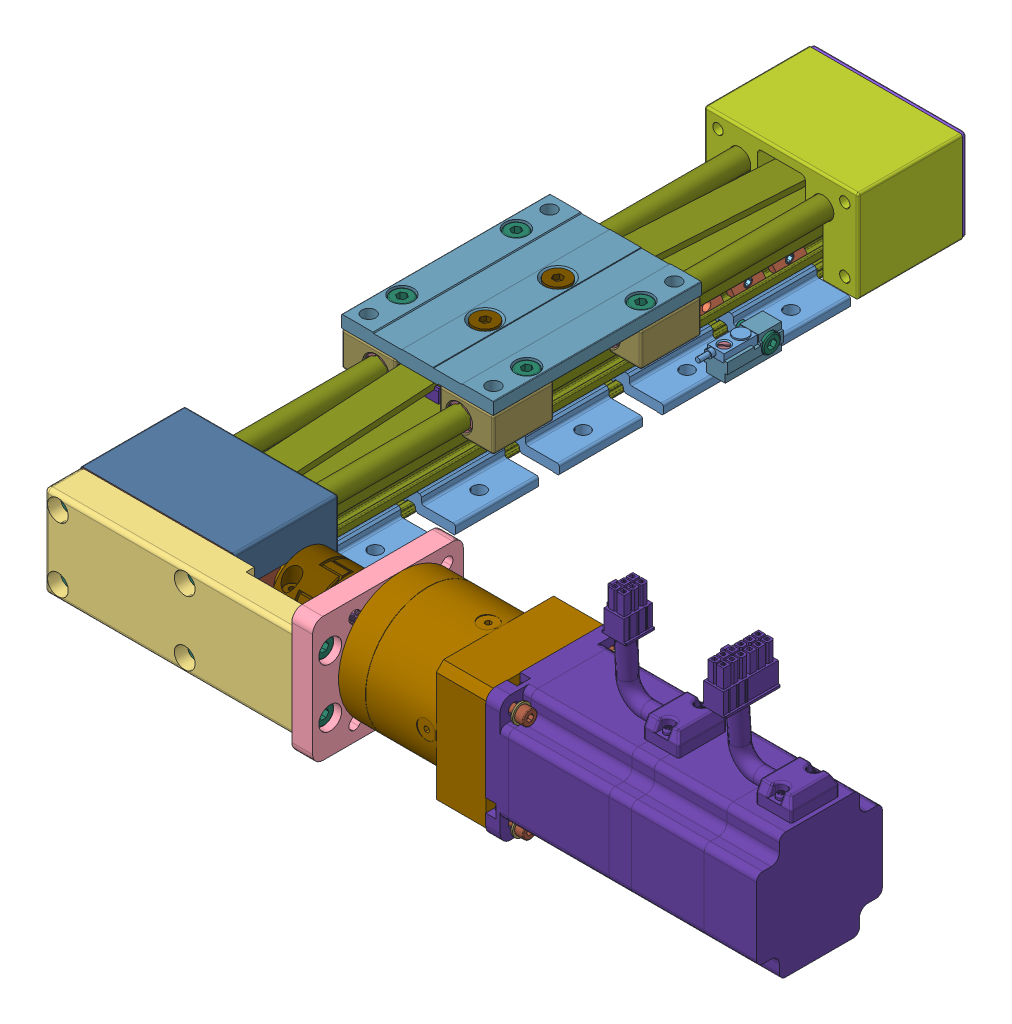
SolidWorks assembly Z Axis, configuration Default. Lengths in mm.
Overall size (331.51 109.68 369.54).
123 component instances, 38 part files, 0 mates.
Components (placement in the parent):
- D00684285.STEP-1: D00684285.STEP [Default] at origin size (331.51 109.68 369.54)
  - D00424608.iam.STEP-1: D00424608.iam.STEP [Default] at (0 0 52) x (-1 0 0) z (0 0 -1) size (74 44 56)
    - D00418189.iam.STEP-1: D00418189.iam.STEP [Default] at (0 22 30) x (-1 0 0) z (0 0 1) size (71 40 33.5)
      - D00160580.ipt.STEP-1: D00160580.ipt.STEP [Default] x (0 0 -1) z (-1 0 0) size (23 23 67.7)
      - D00129954.ipt.STEP-1: D00129954.ipt.STEP [Default] at (-25.5 0 0) x (0 1 0) z (-1 0 0) size (40 30 10)
      - D00129954.ipt.STEP-2: D00129954.ipt.STEP [Default] at (25.5 0 0) x (0 -1 0) z (1 0 0) size (40 30 10)
      - D00130409.ipt.STEP-1: D00130409.ipt.STEP [Default] at (-33.5 0 0) x (0 0 1) z (1 0 0) size (26 26 8)
      - D00130409.ipt.STEP-2: D00130409.ipt.STEP [Default] at (33.5 0 0) x (0 0 -1) z (-1 0 0) size (26 26 8)
      - D00130495.ipt.STEP-1: D00130495.ipt.STEP [Default] at (30.5 -15.5 -15) x (0 0 1) z (-1 0 0) size (23.5 8.5 8.5)
      - D00130495.ipt.STEP-2: D00130495.ipt.STEP [Default] at (-30.5 -15.5 -15) x (0 0 1) z (-1 0 0) size (23.5 8.5 8.5)
      - D00130495.ipt.STEP-3: D00130495.ipt.STEP [Default] at (-30.5 15.5 -15) x (0 0 1) z (-1 0 0) size (23.5 8.5 8.5)
      - D00130495.ipt.STEP-4: D00130495.ipt.STEP [Default] at (30.5 15.5 -15) x (0 0 1) z (1 0 0) size (23.5 8.5 8.5)
      - D00111820.ipt.STEP-1: D00111820.ipt.STEP [Default] at (-30.5 15.5 6.5896) x (0 0 1) z (1 0 0) size (5 5 5)
      - D00111820.ipt.STEP-2: D00111820.ipt.STEP [Default] at (-30.5 -15.5 6.5896) x (0 0 1) z (-1 0 0) size (5 5 5)
      - D00111820.ipt.STEP-3: D00111820.ipt.STEP [Default] at (30.5 -15.5 6.5896) x (0 0 1) z (-1 0 0) size (5 5 5)
      - D00111820.ipt.STEP-4: D00111820.ipt.STEP [Default] at (30.5 15.5 6.5896) x (0 0 1) z (-1 0 0) size (5 5 5)
    - D00129171.ipt.STEP-1: D00129171.ipt.STEP [Default] at (15 23.25 12) x (0 0 -1) z (1 0 0) size (18.8 7 7)
    - D00129171.ipt.STEP-2: D00129171.ipt.STEP [Default] at (-15 23.25 12) x (0 0 -1) z (1 0 0) size (18.8 7 7)
    - D00131296.ipt.STEP-1: D00131296.ipt.STEP [Default] x (-1 0 0) z (0 0 -1) size (74 44 50)
    - SAXT-104002.STEP-1: SAXT-104002.STEP [Default] at (0 22 52) x (-1 0 0) z (0 0 -1) size (74 44 7)
  - D00419202.iam.STEP-1: D00419202.iam.STEP [Default] at (0 0 302) size (94 44 56)
    - D00417520.iam.STEP-1: D00417520.iam.STEP [Default] at (0 22 25) x (-1 0 0) z (0 0 1) size (92.5 40 30)
      - D00130409.ipt.STEP-1: D00130409.ipt.STEP [Default] at (-25.5 0 0) x (0 -0.119291 0.992859) z (-1 0 0) size (26 26 8)
      - D00130409.ipt.STEP-2: D00130409.ipt.STEP [Default] at (33.5 0 0) x (0 0 -1) z (-1 0 0) size (26 26 8)
      - D00129954.ipt.STEP-1: D00129954.ipt.STEP [Default] at (-25.5 0 0) x (0 1 0) z (-1 0 0) size (40 30 10)
      - D00129954.ipt.STEP-2: D00129954.ipt.STEP [Default] at (25.5 0 0) x (0 -1 0) z (1 0 0) size (40 30 10)
      - D00160618.ipt.STEP-1: D00160618.ipt.STEP [Default] x (0 0 1) z (-1 0 0) size (23 23 90.85)
    - D00129171.ipt.STEP-1: D00129171.ipt.STEP [Default] at (15 23.25 12) x (0 0 -1) z (1 0 0) size (18.8 7 7)
    - D00129171.ipt.STEP-2: D00129171.ipt.STEP [Default] at (-15 23.25 12) x (0 0 -1) z (1 0 0) size (18.8 7 7)
    - D00130495.ipt.STEP-1: D00130495.ipt.STEP [Default] at (-30.5 6.5 0) x (0 0 1) z (-1 0 0) size (23.5 8.5 8.5)
    - D00130495.ipt.STEP-2: D00130495.ipt.STEP [Default] at (30.5 6.5 0) x (0 0 1) z (-1 0 0) size (23.5 8.5 8.5)
    - D00131302.ipt.STEP-1: D00131302.ipt.STEP [Default] x (-1 0 0) z (0 0 -1) size (74 44 50)
    - SAXT-104002_1.STEP-1: SAXT-104002_1.STEP [Default] at (0 22 52) x (-1 0 0) z (0 0 -1) size (74 44 24.04)
  - D00132325.iam.STEP-1: D00132325.iam.STEP [Default] at (0 30 177) size (73 22.56 100)
    - D00065372.iam.STEP-1: D00065372.iam.STEP [Default] at (-20 0 -35.5) size (26 17.3 29)
      - D00065332.ipt.STEP-1: D00065332.ipt.STEP [Default] at origin size (26 16.5 29)
      - D00346501.ipt.STEP-1: D00346501.ipt.STEP [Default] x (0.866025 0.5 0) z (0 0 1) size (13.08 12.43 28)
    - D00065372.iam.STEP-2: D00065372.iam.STEP [Default] at (-20 0 35.5) size (26 17.3 29)
      - D00065332.ipt.STEP-1: D00065332.ipt.STEP [Default] at origin size (26 16.5 29)
      - D00346501.ipt.STEP-1: D00346501.ipt.STEP [Default] x (0.866025 0.5 0) z (0 0 1) size (13.08 12.43 28)
    - D00065372.iam.STEP-3: D00065372.iam.STEP [Default] at (20 0 -35.5) x (-1 0 0) z (0 0 -1) size (26 17.3 29)
      - D00065332.ipt.STEP-1: D00065332.ipt.STEP [Default] at origin size (26 16.5 29)
      - D00346501.ipt.STEP-1: D00346501.ipt.STEP [Default] x (0.866025 0.5 0) z (0 0 1) size (13.08 12.43 28)
    - D00065372.iam.STEP-4: D00065372.iam.STEP [Default] at (20 0 35.5) x (-1 0 0) z (0 0 -1) size (26 17.3 29)
      - D00065332.ipt.STEP-1: D00065332.ipt.STEP [Default] at origin size (26 16.5 29)
      - D00346501.ipt.STEP-1: D00346501.ipt.STEP [Default] x (0.866025 0.5 0) z (0 0 1) size (13.08 12.43 28)
    - D00132323.ipt.STEP-1: D00132323.ipt.STEP [Default] at (0 9 0) size (73 6.52 100)
    - D00094049.ipt.STEP-1: D00094049.ipt.STEP [Default] at (30 10.5 27.5) x (0 -1 0) z (-0.000617 0 1) size (20 10 10)
    - D00094049.ipt.STEP-2: D00094049.ipt.STEP [Default] at (30 10.5 -27.5) x (0 -1 0) z (-0.000617 0 1) size (20 10 10)
    - D00094049.ipt.STEP-3: D00094049.ipt.STEP [Default] at (-30 10.5 27.5) x (0 -1 0) z (-0.000617 0 1) size (20 10 10)
    - D00094049.ipt.STEP-4: D00094049.ipt.STEP [Default] at (-30 10.5 -27.5) x (0 -1 0) z (-0.000617 0 1) size (20 10 10)
    - eBom-prt15.STEP-1: eBom-prt15.STEP [Default] at origin
  - D00506371.STEP-1: D00506371.STEP [Default] at (0 22 177) size (20.04 32.95 325.65)
    - D00506373.STEP-1: D00506373.STEP [Default] at origin size (16 26.8 325.65)
    - D00234495.ipt.STEP-1: D00234495.ipt.STEP [Default] at (0 9.875 -30) x (0 0 -1) z (1 0 0) size (40.02 8.02 20.02)
    - D00234495.ipt.STEP-2: D00234495.ipt.STEP [Default] at (0 9.875 30) x (0 0 1) z (-1 0 0) size (40.02 8.02 20.02)
    - D00133498.ipt.STEP-1: D00133498.ipt.STEP [Default] at (0 22.625 -17.5) x (0 -1 0) z (-0.999973 0 -0.007405) size (16 11.34 11.34)
    - D00133498.ipt.STEP-2: D00133498.ipt.STEP [Default] at (0 22.625 17.5) x (0 -1 0) z (-0.997414 0 0.071866) size (16 11.34 11.34)
  - D00308503.iam.STEP-1: D00308503.iam.STEP [Default] at (0 0 57) x (0 1 0) z (0 0 1) size (19.75 76.42 240)
    - D00308504.ipt.STEP-1: D00308504.ipt.STEP [Default] at (0.2 -12.5145 40) x (0 1 0) z (0 0 -1) size (27.65 8.9 40)
    - D00308504.ipt.STEP-2: D00308504.ipt.STEP [Default] at (0.2 12.5145 0) x (0 -1 0) z (0 0 1) size (27.65 8.9 40)
    - D00308504.ipt.STEP-3: D00308504.ipt.STEP [Default] at (0.2 -12.5145 90) x (0 1 0) z (0 0 -1) size (27.65 8.9 40)
    - D00308504.ipt.STEP-4: D00308504.ipt.STEP [Default] at (0.2 12.5145 50) x (0 -1 0) z (0 0 1) size (27.65 8.9 40)
    - D00308504.ipt.STEP-5: D00308504.ipt.STEP [Default] at (0.2 -12.5145 140) x (0 1 0) z (0 0 -1) size (27.65 8.9 40)
    - D00308504.ipt.STEP-6: D00308504.ipt.STEP [Default] at (0.2 12.5145 100) x (0 -1 0) z (0 0 1) size (27.65 8.9 40)
    - D00308504.ipt.STEP-7: D00308504.ipt.STEP [Default] at (0.2 -12.5145 190) x (0 1 0) z (0 0 -1) size (27.65 8.9 40)
    - D00308504.ipt.STEP-8: D00308504.ipt.STEP [Default] at (0.2 12.5145 150) x (0 -1 0) z (0 0 1) size (27.65 8.9 40)
    - D00308504.ipt.STEP-9: D00308504.ipt.STEP [Default] at (0.2 -12.5145 240) x (0 1 0) z (0 0 -1) size (27.65 8.9 40)
    - D00308504.ipt.STEP-10: D00308504.ipt.STEP [Default] at (0.2 12.5145 200) x (0 -1 0) z (0 0 1) size (27.65 8.9 40)
    - D00119001.ipt.STEP-1: D00119001.ipt.STEP [Default] at (15.25 -18.4 9.4087) x (0 0 -1) z (0 1 0) size (19.01 9 4)
    - D00119001.ipt.STEP-2: D00119001.ipt.STEP [Default] at (15.25 14.4 9.4087) x (0 0 -1) z (0 1 0) size (19.01 9 4)
    - D00119001.ipt.STEP-3: D00119001.ipt.STEP [Default] at (15.25 -18.4 29.4087) x (0 0 -1) z (0 1 0) size (19.01 9 4)
    - D00119001.ipt.STEP-4: D00119001.ipt.STEP [Default] at (15.25 14.4 29.4087) x (0 0 -1) z (0 1 0) size (19.01 9 4)
    - D00119001.ipt.STEP-5: D00119001.ipt.STEP [Default] at (15.25 -18.4 49.4087) x (0 0 -1) z (0 1 0) size (19.01 9 4)
    - D00119001.ipt.STEP-6: D00119001.ipt.STEP [Default] at (15.25 14.4 49.4087) x (0 0 -1) z (0 1 0) size (19.01 9 4)
    - D00119001.ipt.STEP-7: D00119001.ipt.STEP [Default] at (15.25 -18.4 69.4087) x (0 0 -1) z (0 1 0) size (19.01 9 4)
    - D00119001.ipt.STEP-8: D00119001.ipt.STEP [Default] at (15.25 14.4 69.4087) x (0 0 -1) z (0 1 0) size (19.01 9 4)
    - D00111820.ipt.STEP-1: D00111820.ipt.STEP [Default] at (15.25 13.4 9.4087) x (0 1 0) z (-0.18197 0 -0.983304) size (5 5 5)
    - D00111820.ipt.STEP-2: D00111820.ipt.STEP [Default] at (15.25 -13.4 9.4087) x (0 -1 0) z (0.628801 0 0.777566) size (5 5 5)
    - D00111820.ipt.STEP-3: D00111820.ipt.STEP [Default] at (15.25 13.4 29.4087) x (0 1 0) z (-0.18197 0 -0.983304) size (5 5 5)
    - D00111820.ipt.STEP-4: D00111820.ipt.STEP [Default] at (15.25 -13.4 29.4087) x (0 -1 0) z (0.628801 0 0.777566) size (5 5 5)
  - D00423744.iam.STEP-1: D00423744.iam.STEP [Default] at (30 22 342) size (138 60 72.54)
    - D00206252.ipt.STEP-1: D00206252.ipt.STEP [Default] at origin size (119 44 27.54)
    - D00210016.ipt.STEP-1: D00210016.ipt.STEP [Default] at (52 0 -15) x (0 -1 0) z (1 0 0) size (60 72.5 10)
    - D00094049.ipt.STEP-1: D00094049.ipt.STEP [Default] at (55 14 19) x (-1 0 0) z (0 0 -1) size (20 10 10)
    - D00095471.ipt.STEP-1: D00095471.ipt.STEP [Default] at (49.6 14 19) x (0 -1 0) z (0 0 -1) size (8 9.2 8)
    - D00094049.ipt.STEP-2: D00094049.ipt.STEP [Default] at (55 -14 19) x (-1 0 0) z (0 0 -1) size (20 10 10)
    - D00095471.ipt.STEP-2: D00095471.ipt.STEP [Default] at (49.6 -14 19) x (0 -1 0) z (0 0 -1) size (8 9.2 8)
    - D00206265.ipt.STEP-1: D00206265.ipt.STEP [Default] at (-60.5 15.5 18) x (0 0 -1) z (1 0 0) size (34.25 10 10)
    - D00206265.ipt.STEP-2: D00206265.ipt.STEP [Default] at (-60.5 -15.5 18) x (0 0 -1) z (1 0 0) size (34.25 10 10)
    - D00206265.ipt.STEP-3: D00206265.ipt.STEP [Default] at (0.5 15.5 18) x (0 0 -1) z (1 0 0) size (34.25 10 10)
    - D00206265.ipt.STEP-4: D00206265.ipt.STEP [Default] at (0.5 -15.5 18) x (0 0 -1) z (1 0 0) size (34.25 10 10)
    - D00095475.ipt.STEP-1: D00095475.ipt.STEP [Default] at (51 17.6777 -32.6777) size (1 10 10)
    - D00130495.ipt.STEP-1: D00130495.ipt.STEP [Default] at (51 17.6777 -32.6777) size (23.5 8.5 8.5)
    - D00025763.ipt.STEP-1: D00025763.ipt.STEP [Default] at (51 17.6777 -32.6777) size (21 8.5 8.5)
    - D00095475.ipt.STEP-2: D00095475.ipt.STEP [Default] at (51 17.6777 2.6777) x (1 0 0) z (0 -1 0) size (1 10 10)
    - D00130495.ipt.STEP-2: D00130495.ipt.STEP [Default] at (51 17.6777 2.6777) x (1 0 0) z (0 -1 0) size (23.5 8.5 8.5)
    - D00025763.ipt.STEP-2: D00025763.ipt.STEP [Default] at (51 17.6777 2.6777) x (1 0 0) z (0 -1 0) size (21 8.5 8.5)
    - D00095475.ipt.STEP-3: D00095475.ipt.STEP [Default] at (51 -17.6777 2.6777) x (1 0 0) z (0 0 -1) size (1 10 10)
    - D00130495.ipt.STEP-3: D00130495.ipt.STEP [Default] at (51 -17.6777 2.6777) x (1 0 0) z (0 0 -1) size (23.5 8.5 8.5)
    - D00025763.ipt.STEP-3: D00025763.ipt.STEP [Default] at (51 -17.6777 2.6777) x (1 0 0) z (0 0 -1) size (21 8.5 8.5)
    - D00095475.ipt.STEP-4: D00095475.ipt.STEP [Default] at (51 -17.6777 -32.6777) x (1 0 0) z (0 1 0) size (1 10 10)
    - D00130495.ipt.STEP-4: D00130495.ipt.STEP [Default] at (51 -17.6777 -32.6777) x (1 0 0) z (0 1 0) size (23.5 8.5 8.5)
    - D00025763.ipt.STEP-4: D00025763.ipt.STEP [Default] at (51 -17.6777 -32.6777) x (1 0 0) z (0 1 0) size (21 8.5 8.5)
  - D00439874.iam.STEP-1: D00439874.iam.STEP [Default] at (92 22 327) x (0 0 1) z (-1 0 0) size (60.02 60.04 120.8)
    - D00376785.ipt.STEP-1: D00376785.ipt.STEP [Default] at origin size (60.02 60.04 106)
    - D00474705.ipt.STEP-1: D00474705.ipt.STEP [Default] at (0 0 -48) x (0 1 0) z (0 0 -1) size (13.95 14 20.03)
    - D00109352.ipt.STEP-1: D00109352.ipt.STEP [Default] at (-23.582 23.582 -81.8) x (0 0 1) z (-1 0 0) size (16 7 7)
    - D00109352.ipt.STEP-2: D00109352.ipt.STEP [Default] at (23.582 23.582 -81.8) x (0 0 1) z (-1 0 0) size (16 7 7)
    - D00109352.ipt.STEP-3: D00109352.ipt.STEP [Default] at (-23.582 -23.582 -81.8) x (0 0 1) z (-1 0 0) size (16 7 7)
    - D00109352.ipt.STEP-4: D00109352.ipt.STEP [Default] at (23.582 -23.582 -81.8) x (0 0 1) z (-1 0 0) size (16 7 7)
    - D00100520.ipt.STEP-1: D00100520.ipt.STEP [Default] at (-23.582 23.582 -81.8) x (0 0 1) z (1 0 0) size (0.8 9 9)
    - D00100520.ipt.STEP-2: D00100520.ipt.STEP [Default] at (23.582 23.582 -81.8) x (0 0 1) z (1 0 0) size (0.8 9 9)
    - D00100520.ipt.STEP-3: D00100520.ipt.STEP [Default] at (-23.582 -23.582 -81.8) x (0 0 1) z (1 0 0) size (0.8 9 9)
    - D00100520.ipt.STEP-4: D00100520.ipt.STEP [Default] at (23.582 -23.582 -81.8) x (0 0 1) z (1 0 0) size (0.8 9 9)
  - D00265100.iam.STEP-1: D00265100.iam.STEP [Default] at (45.4 15.25 127.4087) x (-1 0 0) z (0 0 -1) size (15.5 12.2 27)
    - D00177454.ipt.STEP-1: D00177454.ipt.STEP [Default] at (1.5 5 4) x (0 -1 0) z (0.788943 0 -0.614466) size (10 5.6 5.54)
    - D00177453.ipt.STEP-1: D00177453.ipt.STEP [Default] at origin size (11 12.2 27)
    - D00129169.ipt.STEP-1: D00129169.ipt.STEP [Default] at (-1 0 21) size (15.5 8.5 8.5)
  - D00316386.STEP-1: D00316386.STEP [Default] at (0 0 42) size (50 35 270)
  - D00480302.ipt.STEP-1: D00480302.ipt.STEP [Default] at (163 22 327) x (0 0 1) z (-1 0 0) size (60.5 109.68 151.3)
  - D00416362.ipt.STEP-1: D00416362.ipt.STEP [Default] at (61 22 327) x (0 0 -1) z (1 0 0) size (32.02 32.01 32)
  - D00177460.ipt.STEP-1: D00177460.ipt.STEP [Default] at (43.9 16.75 111.4087) x (-1 0 0) z (0 1 0) size (8 23 4.7)
